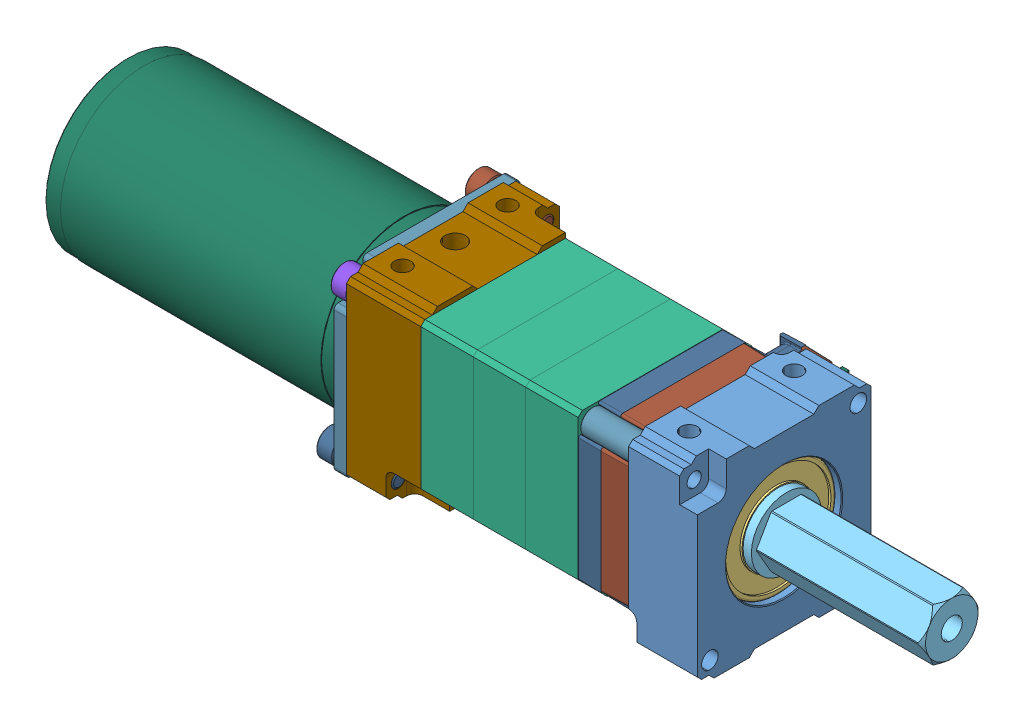
SolidWorks assembly BAG Motor with Encoder, configuration Default. Lengths in mm.
Overall size (201 62.23 62.23).
60 component instances, 52 part files, 12 mates.
Components (placement in the parent):
- Subassembly for BAG Motor with Encoder-1: Subassembly for BAG Motor with Encoder [Default] at (-51.0813 1.3878 0) size (64.12 44.45 42)
  - Part1 - outer gearbox to encoder-1: Part1 - outer gearbox to encoder [Default] at (82.1813 20.8372 0) x (0 -1 0) z (-1 0 0) size (44.45 42 18.12)
  - Part2 - outer ring 1-1: Part2 - outer ring 1 [Default] at (88.8815 20.8372 0) x (1 0 0) z (0 -0.092627 0.995701) size (7 28 28)
  - Part3 - outer ring 2-1: Part3 - outer ring 2 [Default] at (96.8815 20.8372 0) size (7 28 28)
  - Part4 - miscellaneous weird ring-1: Part4 - miscellaneous weird ring [Default] at (96.1013 20.9124 -0.342) x (0 0.56703 0.823697) z (0 -0.823697 0.56703) size (28.51 4.98 30.18)
  - Part5 - 0.5 inch hex shaft-1: Part5 - 0.5 inch hex shaft [Default] at (96.1291 20.8372 0) x (0 -1 0) z (1 0 0) size (17 17 64.12)
  - Part6 - hex shaft collar-1: Part6 - hex shaft collar [Default] at (87.9767 20.8372 0) x (1 0 0) z (0 -0.017452 0.999848) size (1 19.6 17.4)
- Part7 - ring gear screw 1-1: Part7 - ring gear screw 1 [Default] at (-30.7 4.725 -17.5) x (0 0.997447 0.071411) z (0 -0.071411 0.997447) size (6.73 48.51 6.73)
- Part8 - ring gear screw 2-2: Part8 - ring gear screw 2 [Default] at (-30.7 39.725 17.5) x (0 0.005929 0.999982) z (0 -0.999982 0.005929) size (6.73 48.51 6.73)
- Part9 - inner gearbox to motor mount-1: Part9 - inner gearbox to motor mount [Default] at (-23.2 22.225 0) x (0 -1 0) z (-1 0 0) size (44.45 42 18)
- Part10 - ring gear screw 3-1: Part10 - ring gear screw 3 [Default] at (-33.7 4.2645 17.9605) x (0 0.33842 -0.940995) z (0 0.940995 0.33842) size (6.73 16.76 6.73)
- Part11 - ring gear screw 4-2: Part11 - ring gear screw 4 [Default] at (-33.7 40.1855 -17.9605) x (0 -0.308932 -0.951084) z (0 0.951084 -0.308932) size (6.73 16.76 6.73)
- Part12 - motor to mount screw 1-1: Part12 - motor to mount screw 1 [Default] at (-30.7 22.225 12.5) x (0 0.5 -0.866025) z (0 -0.866025 -0.5) size (7 14 7)
- Part13 - motor to mount screw 2-2: Part13 - motor to mount screw 2 [Default] at (-30.7 22.225 -12.5) x (0 -0.5 0.866025) z (0 0.866025 0.5) size (7 14 7)
- Part14 - mounting plate-1: Part14 - mounting plate [Default] at (-32.2 22.225 0) x (0 -1 0) z (-1 0 0) size (42 42 4.8)
- Part15 - BAG motor-1: Part15 - BAG motor [Default] at (-33.7 22.225 0) x (0 0 1) z (1 0 0) size (59.07 59.07 84.5)
- Part25 - Gears Assembly-1: Part25 - Gears Assembly [Default] at (-4.6546 22.225 0) x (0 -0.456494 0.889726) z (-1 0 0) size (39.26 38.9 17.4)
  - Part24 - Tier 1 Gear Subassembly - Subassembly-1: Part24 - Tier 1 Gear Subassembly - Subassembly [Default] at origin size (39.26 38.9 12.7)
    - Part17 - Tier 2 Gear Subassembly - Gear Mount Plate-1: Part17 - Tier 2 Gear Subassembly - Gear Mount Plate [Default] at origin size (34.7 34.7 4.7)
    - Part18 - Tier 2 Gear Subassembly - Gear Pin-1: Part18 - Tier 2 Gear Subassembly - Gear Pin [Default] at (0 10.193 3.65) x (0.999813 0.019336 0) z (0 0 1) size (4 4 12)
    - Part19 - Tier 2 Gear Subassembly - Gear Pin 2-2: Part19 - Tier 2 Gear Subassembly - Gear Pin 2 [Default] at (8.691 -5.3258 3.65) size (4 4 12)
    - Part20 - Tier 2 Gear Subassembly - Gear Pin 3-3: Part20 - Tier 2 Gear Subassembly - Gear Pin 3 [Default] at (-8.691 -5.3258 3.65) size (4 4 12)
    - Part21 - Tier 2 Gear Subassembly - Gear 1-1: Part21 - Tier 2 Gear Subassembly - Gear 1 [Default] at (8.691 -5.3258 6.35) x (0.932816 0.360354 0) z (0 0 1) size (16.91 16.92 8)
    - Part22 - Tier 2 Gear Subassembly - Gear 2-2: Part22 - Tier 2 Gear Subassembly - Gear 2 [Default] at (-8.691 -5.3258 6.35) x (-0.932788 -0.360426 0) z (0 0 1) size (16.91 16.92 8)
    - Part23 - Tier 2 Gear Subassembly - Gear 3-3: Part23 - Tier 2 Gear Subassembly - Gear 3 [Default] at (0 10.193 6.35) x (0.893583 0.448898 0) z (0 0 1) size (16.91 16.92 8)
  - Part16 - Tier 1 Gear Subassembly - Middle gear-1: Part16 - Tier 1 Gear Subassembly - Middle gear [Default] at (0 0 6.7) x (0.992772 0.120019 0) z (0 0 1) size (14.49 14.49 12.72)
- Part26 - inner inner gearbox-1: Part26 - inner inner gearbox [Default] at (-6.35 22.225 0) x (0 -1 0) z (1 0 0) size (42 42 14.5)
- Part27 - keyhole-1: Part27 - keyhole [Default] at (-20.046 22.225 0) x (0 -1 0) z (1 0 0) size (18 18 13)
- Part28 - keyhole bolt-1: Part28 - keyhole bolt [Default] at (-25.521 22.225 -6.7835) x (-0.996104 -0.088191 0) z (0 0 -1) size (4.83 4.83 4.9)
- Part29 - keyhole collar-1: Part29 - keyhole collar [Default] at (-24.7818 22.225 0) x (0 0 1) z (0 -1 0) size (8.01 7.5 7.94)
- Part16 - Integrated Encoder-1: Part16 - Integrated Encoder [Default] at (30.9 22.225 0) x (0 0 1) z (-1 0 0) size (58.06 43.13 22.65)
  - Part6 - Tier 1 Subassembly-1: Part6 - Tier 1 Subassembly [Default] at (0 0 2.75) size (53.55 42 11.11)
  - Part7b - Tier 1 Subassembly-1: Part7b - Tier 1 Subassembly [Default] at (0 0 -7.2) x (0 1 0) z (0 0 1) size (42 51.56 9.32)
  - Part9 - Tier 1 Subassembly-1: Part9 - Tier 1 Subassembly [Default] at (0 0 5.95) x (0.660339 0.750968 0) z (0 0 1) size (21.16 21.1 17.1)
  - Part10 - Tier 1 Subassembly-1: Part10 - Tier 1 Subassembly [Default] at (-20.05 0 5.2) x (-0.718289 0.695745 0) z (0 0 1) size (21.07 21.07 4.88)
  - Part11 - Tier 1 Subassembly-1: Part11 - Tier 1 Subassembly [Default] at (-20.05 0 2.2) x (0.307149 -0.951661 0) z (0.951661 0.307149 0) size (5 4 5)
  - Part12 - Tier 1 Subassembly - Chip-1: Part12 - Tier 1 Subassembly - Chip [Default] at (-20.05 0 -2.1252) x (0 1 0) z (-1 0 0) size (15.93 10.15 24.44)
  - Part13 - Integrated Encoder Bearing-1: Part13 - Integrated Encoder Bearing [Default] at (-20.05 0 3.8125) x (-0.99574 0.092202 0) z (0 0 1) size (9.53 9.53 3.17)
    - Part1 - Tier 2 Subassembly - Outer ring-1: Part1 - Tier 2 Subassembly - Outer ring [Default] at origin size (9.53 9.53 3.17)
    - Part2 - Tier 2 Subassembly - Ball Support-1: Part2 - Tier 2 Subassembly - Ball Support [Default] at origin size (7.38 7.38 3.17)
    - Part3 - Tier 2 Subassembly - Ball 1-13: Part3 - Tier 2 Subassembly - Ball 1 [Default] at origin size (1.52 1.52 1.52)
    - Part3 - Tier 2 Subassembly - Ball 2-14: Part3 - Tier 2 Subassembly - Ball 2 [Default] at origin size (1.52 1.52 1.52)
    - Part3 - Tier 2 Subassembly - Ball 3-2: Part3 - Tier 2 Subassembly - Ball 3 [Default] at origin size (1.52 1.52 1.52)
    - Part3 - Tier 2 Subassembly - Ball 4-12: Part3 - Tier 2 Subassembly - Ball 4 [Default] at origin size (1.52 1.52 1.52)
    - Part3 - Tier 2 Subassembly - Ball 5-3: Part3 - Tier 2 Subassembly - Ball 5 [Default] at origin size (1.52 1.52 1.52)
    - Part3 - Tier 2 Subassembly - Ball 6-4: Part3 - Tier 2 Subassembly - Ball 6 [Default] at origin size (1.52 1.52 1.52)
    - Part3 - Tier 2 Subassembly - Ball 7-5: Part3 - Tier 2 Subassembly - Ball 7 [Default] at origin size (1.52 1.52 1.52)
    - Part3 - Tier 2 Subassembly - Ball 8-6: Part3 - Tier 2 Subassembly - Ball 8 [Default] at origin size (1.52 1.52 1.52)
    - Part3 - Tier 2 Subassembly - Ball 9-9: Part3 - Tier 2 Subassembly - Ball 9 [Default] at origin size (1.52 1.52 1.52)
    - Part3 - Tier 2 Subassembly - Ball 10-7: Part3 - Tier 2 Subassembly - Ball 10 [Default] at origin size (1.52 1.52 1.52)
    - Part3 - Tier 2 Subassembly - Ball 11-10: Part3 - Tier 2 Subassembly - Ball 11 [Default] at origin size (1.52 1.52 1.52)
    - Part3 - Tier 2 Subassembly - Ball 12-11: Part3 - Tier 2 Subassembly - Ball 12 [Default] at origin size (1.52 1.52 1.52)
    - Part4 - Tier 2 Subassembly - Bearing Case 1-1: Part4 - Tier 2 Subassembly - Bearing Case 1 [Default] at origin size (8.5 8.5 0.75)
    - Part5 - Tier 2 Subassembly - Bearing Case 2-12: Part5 - Tier 2 Subassembly - Bearing Case 2 [Default] at origin size (8.5 8.5 0.75)
  - Part13 - Tier 1 Subassembly-1: Part13 - Tier 1 Subassembly [Default] at (17.5 17.5 -0.85) x (-0.867641 0.497191 0) z (0 0 1) size (5.9 5.9 12.7)
  - Part13 - Tier 1 Subassembly-2: Part13 - Tier 1 Subassembly [Default] at (-17.5 -17.5 -0.85) x (0.825154 -0.564908 0) z (0 0 1) size (5.9 5.9 12.7)
  - Part14 - Tier 1 Subassembly-1: Part14 - Tier 1 Subassembly [Default] at (-16.45 0 -5.2) x (0 1 0) z (0 0 1) size (6 10.71 3.56)
  - Part15 - Tier 1 Subassembly-1: Part15 - Tier 1 Subassembly [Default] at (-20.05 0 -1.02) x (0 1 0) z (0 0 1) size (23.4 21.71 4.21)
- Part26 - inner inner gearbox-2: Part26 - inner inner gearbox [Default] at (6.35 22.225 0) x (0 -1 0) z (1 0 0) size (42 42 14.5)
- Part26 - inner inner gearbox-3: Part26 - inner inner gearbox [Default] at (19.05 22.225 0) x (0 -1 0) z (1 0 0) size (42 42 14.5)
Mates (geometry in assembly coordinates):
- Concentric2: concentric aligned: cylinder of Part7 - ring gear screw 1-1 through (13.75 4.725 -17.5) axis (-1 0 0) radius 2.0828; cylinder of Part16 - Integrated Encoder-1/Part13 - Tier 1 Subassembly-2 through (24.3738 4.725 -17.5) axis (-1 0 0) radius 2.2479
- Concentric8: concentric aligned: cylinder of Part8 - ring gear screw 2-2 through (13.75 39.725 17.5) axis (-1 0 0) radius 2.0828; cylinder of Part16 - Integrated Encoder-1/Part13 - Tier 1 Subassembly-1 through (24.3738 39.725 17.5) axis (-1 0 0) radius 2.2479
- Concentric9: concentric anti-aligned: cylinder of Subassembly for BAG Motor with Encoder-1/Part1 - outer gearbox to encoder-1 through (49.961 39.725 17.5) axis (1 0 0) radius 1.7272; cylinder of Part8 - ring gear screw 2-2 through (13.75 39.725 17.5) axis (-1 0 0) radius 2.0828
- Concentric10: concentric anti-aligned: cylinder of Subassembly for BAG Motor with Encoder-1/Part1 - outer gearbox to encoder-1 through (49.961 4.725 -17.5) axis (1 0 0) radius 1.7272; cylinder of Part7 - ring gear screw 1-1 through (13.75 4.725 -17.5) axis (-1 0 0) radius 2.0828
- Coincident9: coincident anti-aligned: plane of Subassembly for BAG Motor with Encoder-1/Part1 - outer gearbox to encoder-1 through (36.1 2.225 0) normal (-1 0 0); plane of Part16 - Integrated Encoder-1/Part7b - Tier 1 Subassembly-1 through (36.1 22.225 0) normal (1 0 0)
- Coincident10: coincident aligned: plane of Part26 - inner inner gearbox-1 through (0 1.225 21) normal (0 -1 0); plane of Part26 - inner inner gearbox-2 through (12.7 1.225 21) normal (0 -1 0)
- Coincident11: coincident aligned: plane of Part26 - inner inner gearbox-1 through (0 43.225 21) normal (0 0 1); plane of Part26 - inner inner gearbox-2 through (12.7 43.225 21) normal (0 0 1)
- Coincident12: coincident anti-aligned: plane of Part26 - inner inner gearbox-1 through (0 1.225 -21) normal (1 0 0); plane of Part26 - inner inner gearbox-2 through (0 1.225 -21) normal (-1 0 0)
- Coincident16: coincident anti-aligned: plane of Part26 - inner inner gearbox-2 through (12.7 1.225 -21) normal (1 0 0); plane of Part26 - inner inner gearbox-3 through (12.7 1.225 -21) normal (-1 0 0)
- Concentric12: concentric aligned: circle of Part26 - inner inner gearbox-2; cylinder of Part26 - inner inner gearbox-3 through (25.4 4.725 -17.5) axis (1 0 0) radius 2.1526
- Concentric13: concentric aligned: circle of Part26 - inner inner gearbox-2; cylinder of Part26 - inner inner gearbox-3 through (25.4 39.725 17.5) axis (1 0 0) radius 2.1526
- Coincident19: coincident anti-aligned: plane of Part16 - Integrated Encoder-1/Part6 - Tier 1 Subassembly-1 through (25.4 22.225 0) normal (-1 0 0); plane of Part26 - inner inner gearbox-3 through (25.4 1.225 -21) normal (1 0 0)
